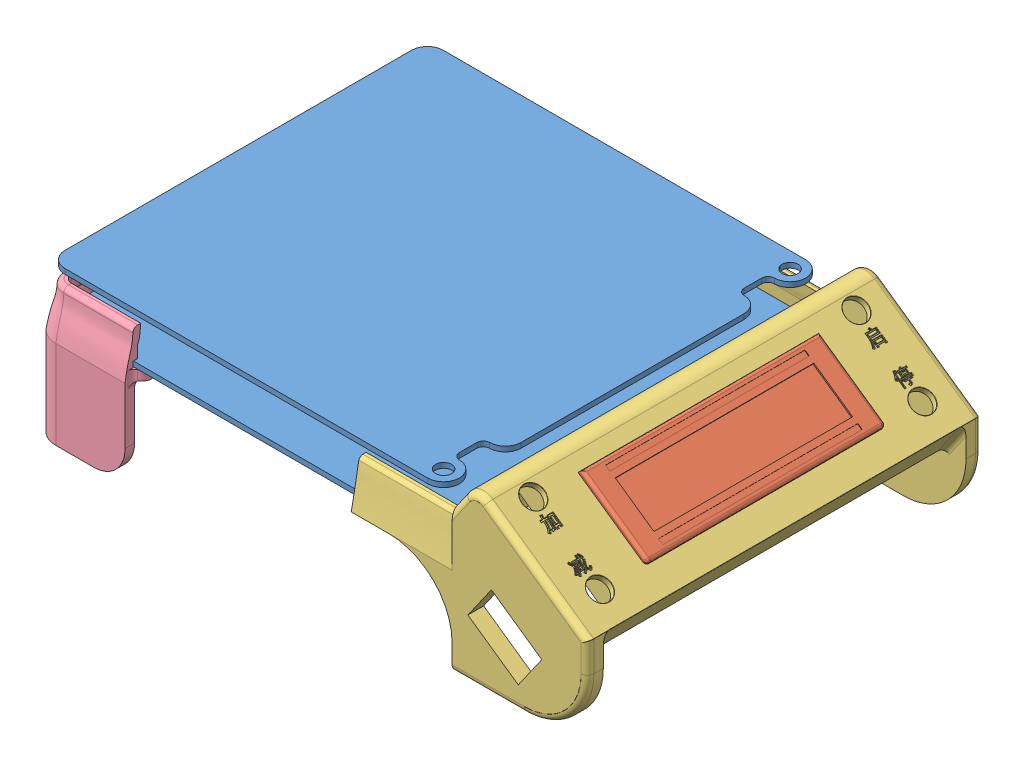
SolidWorks assembly 装配体, configuration 默认. Lengths in mm.
Overall size (183.15 84.67 125.57).
5 component instances, 4 part files, 11 mates.
Components (placement in the parent):
- PCB热床-1: PCB热床 [默认] at (674.8753 2.0312 -453.4606) size (125.06 1.6 119.93)
- PCB热床-2: PCB热床 [默认] at (674.8753 16.5739 -453.4606) size (125.06 1.6 119.93)
- GSH_Bed_V1-1: GSH_Bed_V1 [默认] at (97.7094 -4.2797 82.9817) x (0 0 1) z (-0.573577 -0.819152 0) size (81.5 37.5 20.66)
- 前面板-1: 前面板 [默认] at (68.4572 25.861 62.3317) x (0 0 1) z (-0.573576 -0.819152 0) size (125 77.61 49.02)
- 支架2-2: 支架2 [默认] at (-68.5904 -0.9688 185.3973) x (0 0 -1) z (1 0 0) size (125.4 42.05 32.5)
Mates (geometry in assembly coordinates):
- 重合5: coincident aligned: plane of PCB热床-1 through (-63.4257 3.6312 185.0317) normal (0 0 1); plane of PCB热床-2 through (-63.4257 18.1739 185.0317) normal (0 0 1)
- 重合6: coincident aligned: plane of PCB热床-1 through (56.5743 3.6312 89.7328) normal (1 0 0); plane of PCB热床-2 through (56.5743 18.1739 89.7328) normal (1 0 0)
- 重合13: coincident anti-aligned: plane of GSH_Bed_V1-1 through (69.0622 18.1127 84.1033) normal (0.573576 0.819152 0); plane of 前面板-1 through (65.0157 20.9461 62.3317) normal (-0.573576 -0.819152 0)
- 重合14: coincident anti-aligned: plane of GSH_Bed_V1-1 through (95.4879 -2.222 82.9817) normal (0 0 -1); plane of 前面板-1 through (67.2684 19.3687 82.9817) normal (0 0 1)
- 重合16: coincident: line of GSH_Bed_V1-1 through (97.7094 -4.2797 85.9817) axis (0 0 1); plane of 前面板-1 through (98.8058 -2.714 82.9817) normal (-0.819152 0.573576 0)
- 同心6: concentric aligned: cylinder of PCB热床-1 through (-63.4904 3.6312 70.0973) axis (0 -1 0) radius 5; cylinder of 支架2-2 through (-63.4904 2.0312 70.0973) axis (0 -1 0) radius 5.1
- 重合17: coincident anti-aligned: plane of PCB热床-1 through (-63.4909 2.0312 180.0321) normal (0 -1 0); plane of 支架2-2 through (-63.4904 2.0312 70.0973) normal (0 1 0)
- 平行7: parallel anti-aligned: plane of PCB热床-1 through (-68.4904 3.6312 70.0973) normal (-1 0 0); plane of 支架2-2 through (-68.5904 -0.9688 180.2973) normal (1 0 0)
- 重合24: coincident anti-aligned: plane of PCB热床-1 through (-63.4909 2.0312 180.0321) normal (0 -1 0); plane of 前面板-1 through (26.5743 2.0312 64.6317) normal (0 1 0)
- 重合25: coincident anti-aligned: plane of PCB热床-1 through (-63.4257 3.6312 185.0317) normal (0 0 1); plane of 前面板-1 through (29.5743 -0.9688 185.0317) normal (0 0 -1)
- 距离1: distance = 5 mm aligned: plane of PCB热床-1 through (56.5743 3.6312 89.7328) normal (1 0 0); plane of 前面板-1 through (61.5743 25.861 62.3317) normal (1 0 0)
